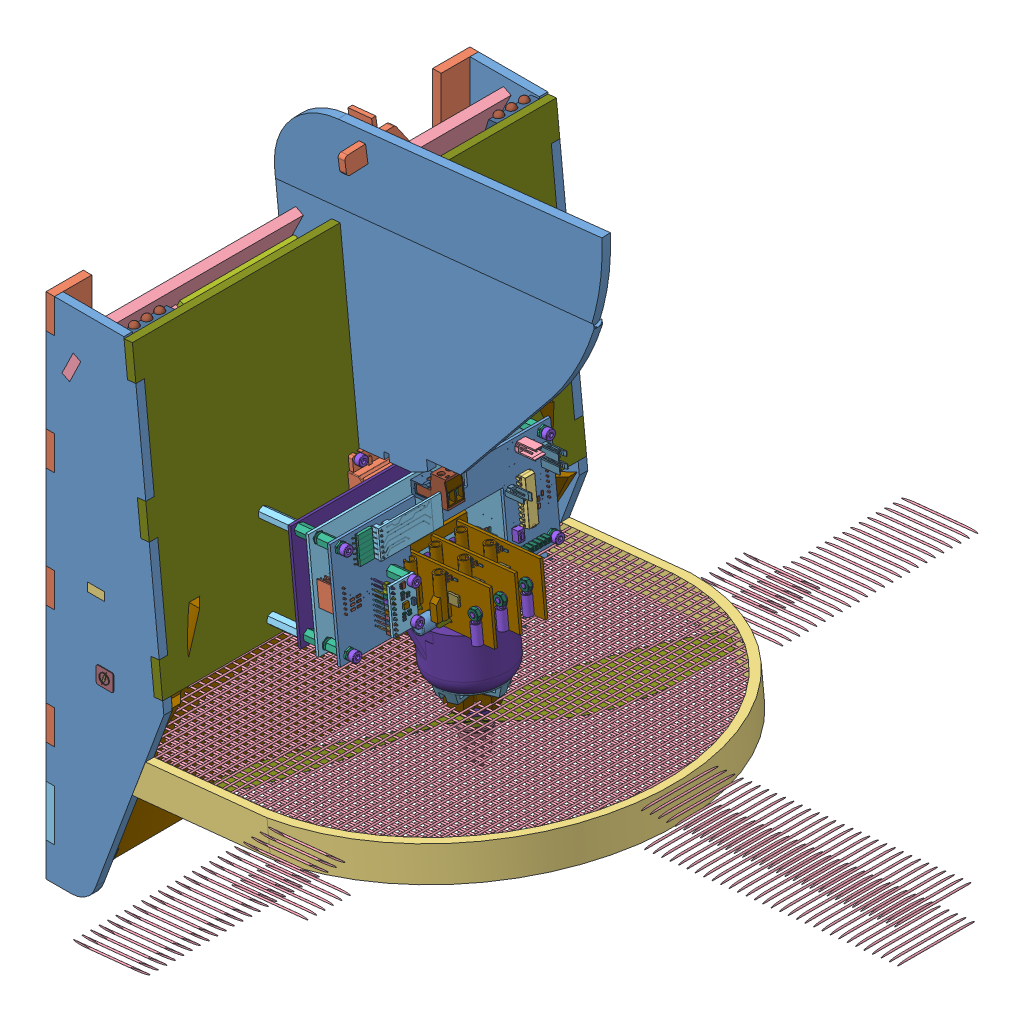
SolidWorks assembly AssTotale, configuration Défaut. Lengths in mm.
Overall size (253.25 376.61 251.6).
1718 component instances, 230 part files, 12 mates.
Components (placement in the parent):
- AssStructSimu-1: AssStructSimu [Défaut] at (-75.9431 -10.8604 24.5323) size (253.25 324.59 251.6)
  - AssBase-1: AssBase [Défaut] at (36.5482 -71.0398 34.0612) size (86.08 302.3 251.6)
    - AssD-1: AssD [Défaut] at (39.0992 31.0201 8.5) size (69.5 300 22)
      - P1-1: P1 [Défaut] at (-95.5819 194.6656 377.5) size (69.5 300 5)
      - P5-1: P5 [Défaut] at (-100.5819 -35.3344 360.5) x (0 1 0) z (1 0 0) size (230 22 5)
    - AssG-1: AssG [Défaut] at (39.0992 31.0201 -236.5) size (69.5 300 22)
      - P1-1: P1 [Défaut] at (-95.5819 194.6656 377.5) size (69.5 300 5)
      - P5-1: P5 [Défaut] at (-95.5819 -35.3344 399.5) x (0 1 0) z (-1 0 0) size (230 22 5)
    - P7-1: P7 [Défaut] at (-1.4828 89.6857 370.5) x (0 0 -1) z (0 -1 0) size (250 54.5 5)
    - P4-1: P4 [Défaut] at (-63.2363 165.9323 386) x (0 0 -1) z (0.898794 -0.438371 0) size (250 60.5 66.27)
    - P3-1: P3 [Défaut] at (-56.4828 -74.3143 146) x (0 0 1) z (-1 0 0) size (250 70 5)
    - P4b-1: P4b [Défaut] at (-58.7423 163.7404 190) x (0 0 1) z (0.438371 0.898794 0) size (152 56 2)
    - battery-1: battery [Défaut] at (-39.0156 204.1861 197.5) x (0 0 1) z (0.898794 -0.438371 0) size (137 43 30)
    - socket head cap screw 4762_din-1: socket head cap screw 4762_din [EN ISO 4762 M3 x 10 - 10N] at (-27.7008 145.2627 193) x (0.438371 0.898794 0) z (0 0 -1) size (13 5.5 5.5)
    - socket head cap screw 4762_din-2: socket head cap screw 4762_din [EN ISO 4762 M3 x 10 - 10N] at (-27.7008 145.2627 339) x (0.438371 0.898794 0) z (-0.791285 0.385936 -0.474259) size (13 5.5 5.5)
    - socket head cap screw 4762_din-3: socket head cap screw 4762_din [EN ISO 4762 M3 x 10 - 10N] at (-42.0815 152.2766 339) x (0.438371 0.898794 0) z (-0.001489 0.000726 -0.999999) size (13 5.5 5.5)
    - socket head cap screw 4762_din-4: socket head cap screw 4762_din [EN ISO 4762 M3 x 10 - 10N] at (-42.0815 152.2766 193) x (0.438371 0.898794 0) z (-0.031331 0.015281 -0.999392) size (13 5.5 5.5)
    - P11-1: P11 [Défaut] at (-57.5734 -73.9703 146.7843) x (0.005072 0 0.999987) z (0.006197 0.999981 -0.000031) size (240 65 164)
    - AssPhare-1: AssPhare [Défaut] at (-52.8518 -67.6977 411) x (0 1 0) z (0 0 -1) size (40.8 8 27.06)
      - piece_led-1: piece_led [Défaut] at (-6.6166 -3.631 25) size (7 8 25)
      - LED 5mm-1: LED 5mm [Valor predeterminado] at (-0.1166 0.369 30) x (0 0 1) z (-1 0 0) size (5.5 6 35.8)
      - LED 5mm-2: LED 5mm [Valor predeterminado] at (-0.1166 0.369 37.5) x (0 0 1) z (-1 0 0) size (5.5 6 35.8)
      - LED 5mm-3: LED 5mm [Valor predeterminado] at (-0.1166 0.369 45) x (0 0 1) z (-1 0 0) size (5.5 6 35.8)
    - AssPhare-2: AssPhare [Défaut] at (-52.8518 -67.6977 196) x (0 1 0) z (0 0 -1) size (40.8 8 27.06)
      - piece_led-1: piece_led [Défaut] at (-6.6166 -3.631 25) size (7 8 25)
      - LED 5mm-1: LED 5mm [Valor predeterminado] at (-0.1166 0.369 30) x (0 0 1) z (-1 0 0) size (5.5 6 35.8)
      - LED 5mm-2: LED 5mm [Valor predeterminado] at (-0.1166 0.369 37.5) x (0 0 1) z (-1 0 0) size (5.5 6 35.8)
      - LED 5mm-3: LED 5mm [Valor predeterminado] at (-0.1166 0.369 45) x (0 0 1) z (-1 0 0) size (5.5 6 35.8)
    - AssLogo-1: AssLogo [Défaut] at (-27.8835 45.1673 148.1054) x (-1 0 0) z (0 0 -1) size (10 10 0.8)
      - logo1-1: logo1 [Défaut] at (-6.5271 -4.4734 6.5054) size (5.8 7.71 0.4)
      - logo2-1: logo2 [Défaut] at (-6.4007 -4.4815 7.1054) size (10 10 0.4)
    - AssLogo-2: AssLogo [Défaut] at (-25.082 45.1673 383.8946) size (10 10 0.8)
      - logo1-1: logo1 [Défaut] at (-6.5271 -4.4734 6.5054) size (5.8 7.71 0.4)
      - logo2-1: logo2 [Défaut] at (-6.4007 -4.4815 7.1054) size (10 10 0.4)
    - support2-1: support2 [Défaut] at (-61.5648 191.7124 276) x (-0.017452 -0.999848 0) z (0.999848 -0.017452 0) size (75 20 10)
    - socket head cap screw 4762_din-5: socket head cap screw 4762_din [EN ISO 4762 M3 x 5 - 5N] at (-61.652 186.7132 269.3333) x (0.999848 -0.017452 0) z (-0.002158 -0.123615 0.992328) size (8 5.5 5.5)
    - socket head cap screw 4762_din-6: socket head cap screw 4762_din [EN ISO 4762 M3 x 5 - 5N] at (-61.652 186.7132 262.6667) x (0.999848 -0.017452 0) z (0 0 1) size (8 5.5 5.5)
    - socket head cap screw 4762_din-7: socket head cap screw 4762_din [EN ISO 4762 M3 x 25 - 18N] at (-55.2963 121.0922 253) x (0 0 1) z (-1 0 0) size (28 5.5 5.5)
    - hex nut style 1 gradeab_din-1: hex nut style 1 gradeab_din [Hexagon Nut ISO 4032 - M3 - W - N] at (-55.2963 121.0922 276) x (-0.923728 -0.383049 0) z (0 0 -1) size (5.5 6.35 2.4)
  - AssToitMot-1: AssToitMot [Défaut] at (-168.5238 43.6961 238.494) x (0 0 -1) z (0.9948 0.101852 0) size (250 207.5 205)
    - AssToit-1: AssToit [Défaut] at (-23.0702 -16.5789 -3.7148) size (250 207.5 205)
      - P8-1: P8 [Défaut] at (-38.4971 122.5921 203.5) size (250 175 5)
      - P12-1: P12 [Défaut] at (-60.4971 -63.4079 265.5) x (1 0 0) z (0 -1 0) size (47.03 76.64 55)
      - P13-1: P13 [Défaut] at (-35.9971 -52.8579 208.5) x (0 0 1) z (-1 0 0) size (64 15.55 5)
      - P10_2-1: P10_2 [Défaut] at (-35.9971 111.5921 171) x (0 0 1) z (-1 0 0) size (188.5 117.6 5)
    - Parallax-Servo_DUMMY-1: Parallax-Servo_DUMMY [Défaut] at (-61.6002 -51.5207 216.6662) x (1 0 0) z (0 1 0) size (20.07 42.67 55.64)
    - socket head cap screw 4762_din-1: socket head cap screw 4762_din [EN ISO 4762 M2.5 x 5 - 5N] at (-51.9272 -76.4868 259.2852) x (0 -1 0) z (-0.546944 0 0.837169) size (7.5 4.5 4.5)
    - socket head cap screw 4762_din-2: socket head cap screw 4762_din [EN ISO 4762 M2.5 x 5 - 5N] at (-61.5672 -76.4868 268.9252) x (0 -1 0) z (-0.546944 0 0.837169) size (7.5 4.5 4.5)
    - socket head cap screw 4762_din-3: socket head cap screw 4762_din [EN ISO 4762 M2.5 x 5 - 5N] at (-71.2072 -76.4868 259.2852) x (0 -1 0) z (-0.546944 0 0.837169) size (7.5 4.5 4.5)
    - socket head cap screw 4762_din-4: socket head cap screw 4762_din [EN ISO 4762 M2.5 x 5 - 5N] at (-61.5672 -76.4868 249.6452) x (0 -1 0) z (-0.546944 0 0.837169) size (7.5 4.5 4.5)
    - AssPhare-1: AssPhare [Défaut] at (8.4328 83.3966 196.1542) x (0 -1 0) z (1 0 0) size (40.8 8 27.06)
      - piece_led-1: piece_led [Défaut] at (-6.6166 -3.631 25) size (7 8 25)
      - LED 5mm-1: LED 5mm [Valor predeterminado] at (-0.1166 0.369 30) x (0 0 1) z (-1 0 0) size (5.5 6 35.8)
      - LED 5mm-2: LED 5mm [Valor predeterminado] at (-0.1166 0.369 37.5) x (0 0 1) z (-1 0 0) size (5.5 6 35.8)
      - LED 5mm-3: LED 5mm [Valor predeterminado] at (-0.1166 0.369 45) x (0 0 1) z (-1 0 0) size (5.5 6 35.8)
    - AssPhare-2: AssPhare [Défaut] at (-206.5672 83.3966 196.1542) x (0 -1 0) z (1 0 0) size (40.8 8 27.06)
      - piece_led-1: piece_led [Défaut] at (-6.6166 -3.631 25) size (7 8 25)
      - LED 5mm-1: LED 5mm [Valor predeterminado] at (-0.1166 0.369 30) x (0 0 1) z (-1 0 0) size (5.5 6 35.8)
      - LED 5mm-2: LED 5mm [Valor predeterminado] at (-0.1166 0.369 37.5) x (0 0 1) z (-1 0 0) size (5.5 6 35.8)
      - LED 5mm-3: LED 5mm [Valor predeterminado] at (-0.1166 0.369 45) x (0 0 1) z (-1 0 0) size (5.5 6 35.8)
    - socket head cap screw 4762_din-5: socket head cap screw 4762_din [EN ISO 4762 M3 x 10 - 10N] at (-67.0672 -22.9368 210.2852) x (0 0 -1) z (1 0 0) size (13 5.5 5.5)
    - socket head cap screw 4762_din-6: socket head cap screw 4762_din [EN ISO 4762 M3 x 10 - 10N] at (-56.0672 -72.9868 210.2852) x (0 0 -1) z (1 0 0) size (13 5.5 5.5)
    - socket head cap screw 4762_din-7: socket head cap screw 4762_din [EN ISO 4762 M3 x 10 - 10N] at (-67.0672 -72.9868 210.2852) x (0 0 -1) z (1 0 0) size (13 5.5 5.5)
    - socket head cap screw 4762_din-8: socket head cap screw 4762_din [EN ISO 4762 M3 x 10 - 10N] at (-56.0672 -22.9368 210.2852) x (0 0 -1) z (1 0 0) size (13 5.5 5.5)
    - hex nut style 1 gradeab_din-1: hex nut style 1 gradeab_din [Hexagon Nut ISO 4032 - M3 - W - N] at (-67.0672 -72.9868 197.3852) x (-0.923728 -0.383049 0) z (0 0 -1) size (5.5 6.35 2.4)
    - hex nut style 1 gradeab_din-2: hex nut style 1 gradeab_din [Hexagon Nut ISO 4032 - M3 - W - N] at (-56.0672 -72.9868 199.7852) size (5.5 6.35 2.4)
    - hex nut style 1 gradeab_din-3: hex nut style 1 gradeab_din [Hexagon Nut ISO 4032 - M3 - W - N] at (-67.0672 -22.9368 199.7852) size (5.5 6.35 2.4)
    - hex nut style 1 gradeab_din-4: hex nut style 1 gradeab_din [Hexagon Nut ISO 4032 - M3 - W - N] at (-56.0672 -22.9368 199.7852) size (5.5 6.35 2.4)
  - AssProtec-1: AssProtec [Défaut] at (86.6746 190.4649 284.6351) x (0 0 -1) z (0.101852 -0.9948 0) size (250 237.46 20)
    - protec3c-1: protec3c [Défaut] at (-140.4261 -87.7568 240) size (250 197 20)
    - AssGrillage-1: AssGrillage [Défaut] at (-370.4609 -132.5428 258.3161) x (0 0 -1) z (1 0 0) size (2.02 237.05 250)
      - barreau-1: barreau [Défaut] at (-1.1839 0.254 200) size (1 1 400)
      - barreau-3: barreau [Défaut] at (-1.1839 5.254 200) size (1 1 400)
      - barreau-4: barreau [Défaut] at (-1.1839 10.254 200) size (1 1 400)
      - barreau-5: barreau [Défaut] at (-1.1839 15.254 200) size (1 1 400)
      - barreau-6: barreau [Défaut] at (-1.1839 20.254 200) size (1 1 400)
      - barreau-7: barreau [Défaut] at (-1.1839 25.254 200) size (1 1 400)
      - barreau-8: barreau [Défaut] at (-1.1839 30.254 200) size (1 1 400)
      - barreau-9: barreau [Défaut] at (-1.1839 35.254 200) size (1 1 400)
      - barreau-10: barreau [Défaut] at (-1.1839 40.254 200) size (1 1 400)
      - barreau-11: barreau [Défaut] at (-1.1839 45.254 200) size (1 1 400)
      - barreau-12: barreau [Défaut] at (-1.1839 50.254 200) size (1 1 400)
      - barreau-13: barreau [Défaut] at (-1.1839 55.254 200) size (1 1 400)
      - barreau-14: barreau [Défaut] at (-1.1839 60.254 200) size (1 1 400)
      - barreau-15: barreau [Défaut] at (-1.1839 65.254 200) size (1 1 400)
      - barreau-16: barreau [Défaut] at (-1.1839 70.254 200) size (1 1 400)
      - barreau-17: barreau [Défaut] at (-1.1839 75.254 200) size (1 1 400)
      - barreau-18: barreau [Défaut] at (-1.1839 80.254 200) size (1 1 400)
      - barreau-19: barreau [Défaut] at (-1.1839 85.254 200) size (1 1 400)
      - barreau-20: barreau [Défaut] at (-1.1839 90.254 200) size (1 1 400)
      - barreau-21: barreau [Défaut] at (-1.1839 95.254 200) size (1 1 400)
      - barreau-22: barreau [Défaut] at (-1.1839 100.254 200) size (1 1 400)
      - barreau-23: barreau [Défaut] at (-1.1839 105.254 200) size (1 1 400)
      - barreau-24: barreau [Défaut] at (-1.1839 110.254 200) size (1 1 400)
      - barreau-25: barreau [Défaut] at (-1.1839 115.254 200) size (1 1 400)
      - barreau-26: barreau [Défaut] at (-1.1839 120.254 200) size (1 1 400)
      - barreau-27: barreau [Défaut] at (-1.1839 125.254 200) size (1 1 400)
      - barreau-28: barreau [Défaut] at (-1.1839 130.254 200) size (1 1 400)
      - barreau-29: barreau [Défaut] at (-1.1839 135.254 200) size (1 1 400)
      - barreau-30: barreau [Défaut] at (-1.1839 140.254 200) size (1 1 400)
      - barreau-31: barreau [Défaut] at (-1.1839 145.254 200) size (1 1 400)
      - barreau-32: barreau [Défaut] at (-1.1839 150.254 200) size (1 1 400)
      - barreau-33: barreau [Défaut] at (-1.1839 155.254 200) size (1 1 400)
      - barreau-34: barreau [Défaut] at (-1.1839 160.254 200) size (1 1 400)
      - barreau-35: barreau [Défaut] at (-1.1839 165.254 200) size (1 1 400)
      - barreau-36: barreau [Défaut] at (-1.1839 170.254 200) size (1 1 400)
      - barreau-37: barreau [Défaut] at (-1.1839 175.254 200) size (1 1 400)
      - barreau-38: barreau [Défaut] at (-1.1839 180.254 200) size (1 1 400)
      - barreau-39: barreau [Défaut] at (-1.1839 185.254 200) size (1 1 400)
      - barreau-40: barreau [Défaut] at (-1.1839 190.254 200) size (1 1 400)
      - barreau-41: barreau [Défaut] at (-1.1839 195.254 200) size (1 1 400)
      - barreau-42: barreau [Défaut] at (-0.1839 -1.5314 598.7823) x (0.998922 0 0.04641) z (0 1 0) size (1 1 400)
      - barreau-43: barreau [Défaut] at (-1.1839 200.254 200) size (1 1 400)
      - barreau-44: barreau [Défaut] at (-1.1839 205.254 200) size (1 1 400)
      - barreau-45: barreau [Défaut] at (-1.1839 210.254 200) size (1 1 400)
      - barreau-46: barreau [Défaut] at (-1.1839 215.254 200) size (1 1 400)
      - barreau-47: barreau [Défaut] at (-1.1839 220.254 200) size (1 1 400)
      - barreau-48: barreau [Défaut] at (-1.1839 225.254 200) size (1 1 400)
      - barreau-49: barreau [Défaut] at (-1.1839 230.254 200) size (1 1 400)
      - barreau-50: barreau [Défaut] at (-1.1839 235.254 200) size (1 1 400)
      - barreau-51: barreau [Défaut] at (-1.1839 240.254 200) size (1 1 400)
      - barreau-52: barreau [Défaut] at (-1.1839 245.254 200) size (1 1 400)
      - barreau-53: barreau [Défaut] at (-1.1839 250.254 200) size (1 1 400)
      - barreau-54: barreau [Défaut] at (-1.1839 255.254 200) size (1 1 400)
      - barreau-55: barreau [Défaut] at (-1.1839 260.254 200) size (1 1 400)
      - barreau-56: barreau [Défaut] at (-1.1839 265.254 200) size (1 1 400)
      - barreau-57: barreau [Défaut] at (-1.1839 270.254 200) size (1 1 400)
      - barreau-58: barreau [Défaut] at (-1.1839 275.254 200) size (1 1 400)
      - barreau-59: barreau [Défaut] at (-1.1839 280.254 200) size (1 1 400)
      - barreau-60: barreau [Défaut] at (-1.1839 285.254 200) size (1 1 400)
      - barreau-61: barreau [Défaut] at (-1.1839 290.254 200) size (1 1 400)
      - barreau-62: barreau [Défaut] at (-1.1839 295.254 200) size (1 1 400)
      - barreau-63: barreau [Défaut] at (-1.1839 300.254 200) size (1 1 400)
      - barreau-64: barreau [Défaut] at (-1.1839 305.254 200) size (1 1 400)
      - barreau-65: barreau [Défaut] at (-1.1839 310.254 200) size (1 1 400)
      - barreau-66: barreau [Défaut] at (-1.1839 315.254 200) size (1 1 400)
      - barreau-67: barreau [Défaut] at (-1.1839 320.254 200) size (1 1 400)
      - barreau-68: barreau [Défaut] at (-1.1839 325.254 200) size (1 1 400)
      - barreau-69: barreau [Défaut] at (-1.1839 330.254 200) size (1 1 400)
      - barreau-70: barreau [Défaut] at (-1.1839 335.254 200) size (1 1 400)
      - barreau-71: barreau [Défaut] at (-1.1839 340.254 200) size (1 1 400)
      - barreau-72: barreau [Défaut] at (-1.1839 345.254 200) size (1 1 400)
      - barreau-73: barreau [Défaut] at (-1.1839 350.254 200) size (1 1 400)
      - barreau-74: barreau [Défaut] at (-1.1839 355.254 200) size (1 1 400)
      - barreau-75: barreau [Défaut] at (-1.1839 360.254 200) size (1 1 400)
      - barreau-76: barreau [Défaut] at (-1.1839 365.254 200) size (1 1 400)
      - barreau-77: barreau [Défaut] at (-1.1839 370.254 200) size (1 1 400)
      - barreau-78: barreau [Défaut] at (-1.1839 375.254 200) size (1 1 400)
      - barreau-79: barreau [Défaut] at (-1.1839 380.254 200) size (1 1 400)
      - barreau-80: barreau [Défaut] at (-1.1839 385.254 200) size (1 1 400)
      - barreau-81: barreau [Défaut] at (-1.1839 390.254 200) size (1 1 400)
      - barreau-82: barreau [Défaut] at (-1.1839 395.254 200) size (1 1 400)
      - barreau-136: barreau [Défaut] at (-0.1839 -1.5314 593.7823) x (0.998922 0 0.04641) z (0 1 0) size (1 1 400)
      - barreau-137: barreau [Défaut] at (-0.1839 -1.5314 588.7823) x (0.998922 0 0.04641) z (0 1 0) size (1 1 400)
      - barreau-138: barreau [Défaut] at (-0.1839 -1.5314 583.7823) x (0.998922 0 0.04641) z (0 1 0) size (1 1 400)
      - barreau-139: barreau [Défaut] at (-0.1839 -1.5314 578.7823) x (0.998922 0 0.04641) z (0 1 0) size (1 1 400)
      - barreau-140: barreau [Défaut] at (-0.1839 -1.5314 573.7823) x (0.998922 0 0.04641) z (0 1 0) size (1 1 400)
      - barreau-141: barreau [Défaut] at (-0.1839 -1.5314 568.7823) x (0.998922 0 0.04641) z (0 1 0) size (1 1 400)
      - barreau-142: barreau [Défaut] at (-0.1839 -1.5314 563.7823) x (0.998922 0 0.04641) z (0 1 0) size (1 1 400)
      - barreau-143: barreau [Défaut] at (-0.1839 -1.5314 558.7823) x (0.998922 0 0.04641) z (0 1 0) size (1 1 400)
      - barreau-144: barreau [Défaut] at (-0.1839 -1.5314 553.7823) x (0.998922 0 0.04641) z (0 1 0) size (1 1 400)
      - barreau-145: barreau [Défaut] at (-0.1839 -1.5314 548.7823) x (0.998922 0 0.04641) z (0 1 0) size (1 1 400)
      - barreau-146: barreau [Défaut] at (-0.1839 -1.5314 543.7823) x (0.998922 0 0.04641) z (0 1 0) size (1 1 400)
      - barreau-147: barreau [Défaut] at (-0.1839 -1.5314 538.7823) x (0.998922 0 0.04641) z (0 1 0) size (1 1 400)
      - barreau-148: barreau [Défaut] at (-0.1839 -1.5314 533.7823) x (0.998922 0 0.04641) z (0 1 0) size (1 1 400)
      - barreau-149: barreau [Défaut] at (-0.1839 -1.5314 528.7823) x (0.998922 0 0.04641) z (0 1 0) size (1 1 400)
      - barreau-150: barreau [Défaut] at (-0.1839 -1.5314 523.7823) x (0.998922 0 0.04641) z (0 1 0) size (1 1 400)
      - barreau-151: barreau [Défaut] at (-0.1839 -1.5314 518.7823) x (0.998922 0 0.04641) z (0 1 0) size (1 1 400)
      - barreau-152: barreau [Défaut] at (-0.1839 -1.5314 513.7823) x (0.998922 0 0.04641) z (0 1 0) size (1 1 400)
      - barreau-153: barreau [Défaut] at (-0.1839 -1.5314 508.7823) x (0.998922 0 0.04641) z (0 1 0) size (1 1 400)
      - barreau-154: barreau [Défaut] at (-0.1839 -1.5314 503.7823) x (0.998922 0 0.04641) z (0 1 0) size (1 1 400)
      - barreau-155: barreau [Défaut] at (-0.1839 -1.5314 498.7823) x (0.998922 0 0.04641) z (0 1 0) size (1 1 400)
      - barreau-156: barreau [Défaut] at (-0.1839 -1.5314 493.7823) x (0.998922 0 0.04641) z (0 1 0) size (1 1 400)
      - barreau-157: barreau [Défaut] at (-0.1839 -1.5314 488.7823) x (0.998922 0 0.04641) z (0 1 0) size (1 1 400)
      - barreau-158: barreau [Défaut] at (-0.1839 -1.5314 483.7823) x (0.998922 0 0.04641) z (0 1 0) size (1 1 400)
      - barreau-159: barreau [Défaut] at (-0.1839 -1.5314 478.7823) x (0.998922 0 0.04641) z (0 1 0) size (1 1 400)
      - barreau-160: barreau [Défaut] at (-0.1839 -1.5314 473.7823) x (0.998922 0 0.04641) z (0 1 0) size (1 1 400)
      - barreau-161: barreau [Défaut] at (-0.1839 -1.5314 468.7823) x (0.998922 0 0.04641) z (0 1 0) size (1 1 400)
      - barreau-162: barreau [Défaut] at (-0.1839 -1.5314 463.7823) x (0.998922 0 0.04641) z (0 1 0) size (1 1 400)
      - barreau-163: barreau [Défaut] at (-0.1839 -1.5314 458.7823) x (0.998922 0 0.04641) z (0 1 0) size (1 1 400)
      - barreau-164: barreau [Défaut] at (-0.1839 -1.5314 453.7823) x (0.998922 0 0.04641) z (0 1 0) size (1 1 400)
      - barreau-165: barreau [Défaut] at (-0.1839 -1.5314 448.7823) x (0.998922 0 0.04641) z (0 1 0) size (1 1 400)
      - barreau-166: barreau [Défaut] at (-0.1839 -1.5314 443.7823) x (0.998922 0 0.04641) z (0 1 0) size (1 1 400)
      - barreau-167: barreau [Défaut] at (-0.1839 -1.5314 438.7823) x (0.998922 0 0.04641) z (0 1 0) size (1 1 400)
      - barreau-168: barreau [Défaut] at (-0.1839 -1.5314 433.7823) x (0.998922 0 0.04641) z (0 1 0) size (1 1 400)
      - barreau-169: barreau [Défaut] at (-0.1839 -1.5314 428.7823) x (0.998922 0 0.04641) z (0 1 0) size (1 1 400)
      - barreau-170: barreau [Défaut] at (-0.1839 -1.5314 423.7823) x (0.998922 0 0.04641) z (0 1 0) size (1 1 400)
      - barreau-171: barreau [Défaut] at (-0.1839 -1.5314 418.7823) x (0.998922 0 0.04641) z (0 1 0) size (1 1 400)
      - barreau-172: barreau [Défaut] at (-0.1839 -1.5314 413.7823) x (0.998922 0 0.04641) z (0 1 0) size (1 1 400)
      - barreau-173: barreau [Défaut] at (-0.1839 -1.5314 408.7823) x (0.998922 0 0.04641) z (0 1 0) size (1 1 400)
      - barreau-174: barreau [Défaut] at (-0.1839 -1.5314 403.7823) x (0.998922 0 0.04641) z (0 1 0) size (1 1 400)
      - barreau-175: barreau [Défaut] at (-0.1839 -1.5314 398.7823) x (0.998922 0 0.04641) z (0 1 0) size (1 1 400)
      - barreau-176: barreau [Défaut] at (-0.1839 -1.5314 393.7823) x (0.998922 0 0.04641) z (0 1 0) size (1 1 400)
      - barreau-177: barreau [Défaut] at (-0.1839 -1.5314 388.7823) x (0.998922 0 0.04641) z (0 1 0) size (1 1 400)
      - barreau-178: barreau [Défaut] at (-0.1839 -1.5314 383.7823) x (0.998922 0 0.04641) z (0 1 0) size (1 1 400)
      - barreau-179: barreau [Défaut] at (-0.1839 -1.5314 378.7823) x (0.998922 0 0.04641) z (0 1 0) size (1 1 400)
      - barreau-180: barreau [Défaut] at (-0.1839 -1.5314 373.7823) x (0.998922 0 0.04641) z (0 1 0) size (1 1 400)
      - barreau-181: barreau [Défaut] at (-0.1839 -1.5314 368.7823) x (0.998922 0 0.04641) z (0 1 0) size (1 1 400)
      - barreau-182: barreau [Défaut] at (-0.1839 -1.5314 363.7823) x (0.998922 0 0.04641) z (0 1 0) size (1 1 400)
      - barreau-183: barreau [Défaut] at (-0.1839 -1.5314 358.7823) x (0.998922 0 0.04641) z (0 1 0) size (1 1 400)
      - barreau-184: barreau [Défaut] at (-0.1839 -1.5314 353.7823) x (0.998922 0 0.04641) z (0 1 0) size (1 1 400)
      - barreau-185: barreau [Défaut] at (-0.1839 -1.5314 348.7823) x (0.998922 0 0.04641) z (0 1 0) size (1 1 400)
      - barreau-186: barreau [Défaut] at (-0.1839 -1.5314 343.7823) x (0.998922 0 0.04641) z (0 1 0) size (1 1 400)
      - barreau-187: barreau [Défaut] at (-0.1839 -1.5314 338.7823) x (0.998922 0 0.04641) z (0 1 0) size (1 1 400)
      - barreau-188: barreau [Défaut] at (-0.1839 -1.5314 333.7823) x (0.998922 0 0.04641) z (0 1 0) size (1 1 400)
      - barreau-189: barreau [Défaut] at (-0.1839 -1.5314 328.7823) x (0.998922 0 0.04641) z (0 1 0) size (1 1 400)
      - barreau-190: barreau [Défaut] at (-0.1839 -1.5314 323.7823) x (0.998922 0 0.04641) z (0 1 0) size (1 1 400)
      - barreau-191: barreau [Défaut] at (-0.1839 -1.5314 318.7823) x (0.998922 0 0.04641) z (0 1 0) size (1 1 400)
      - barreau-192: barreau [Défaut] at (-0.1839 -1.5314 313.7823) x (0.998922 0 0.04641) z (0 1 0) size (1 1 400)
      - barreau-193: barreau [Défaut] at (-0.1839 -1.5314 308.7823) x (0.998922 0 0.04641) z (0 1 0) size (1 1 400)
      - barreau-194: barreau [Défaut] at (-0.1839 -1.5314 303.7823) x (0.998922 0 0.04641) z (0 1 0) size (1 1 400)
      - barreau-195: barreau [Défaut] at (-0.1839 -1.5314 298.7823) x (0.998922 0 0.04641) z (0 1 0) size (1 1 400)
      - barreau-196: barreau [Défaut] at (-0.1839 -1.5314 293.7823) x (0.998922 0 0.04641) z (0 1 0) size (1 1 400)
      - barreau-197: barreau [Défaut] at (-0.1839 -1.5314 288.7823) x (0.998922 0 0.04641) z (0 1 0) size (1 1 400)
      - barreau-198: barreau [Défaut] at (-0.1839 -1.5314 283.7823) x (0.998922 0 0.04641) z (0 1 0) size (1 1 400)
      - barreau-199: barreau [Défaut] at (-0.1839 -1.5314 278.7823) x (0.998922 0 0.04641) z (0 1 0) size (1 1 400)
      - barreau-200: barreau [Défaut] at (-0.1839 -1.5314 273.7823) x (0.998922 0 0.04641) z (0 1 0) size (1 1 400)
      - barreau-201: barreau [Défaut] at (-0.1839 -1.5314 268.7823) x (0.998922 0 0.04641) z (0 1 0) size (1 1 400)
      - barreau-202: barreau [Défaut] at (-0.1839 -1.5314 263.7823) x (0.998922 0 0.04641) z (0 1 0) size (1 1 400)
      - barreau-203: barreau [Défaut] at (-0.1839 -1.5314 258.7823) x (0.998922 0 0.04641) z (0 1 0) size (1 1 400)
      - barreau-204: barreau [Défaut] at (-0.1839 -1.5314 253.7823) x (0.998922 0 0.04641) z (0 1 0) size (1 1 400)
      - barreau-205: barreau [Défaut] at (-0.1839 -1.5314 248.7823) x (0.998922 0 0.04641) z (0 1 0) size (1 1 400)
      - barreau-206: barreau [Défaut] at (-0.1839 -1.5314 243.7823) x (0.998922 0 0.04641) z (0 1 0) size (1 1 400)
      - barreau-207: barreau [Défaut] at (-0.1839 -1.5314 238.7823) x (0.998922 0 0.04641) z (0 1 0) size (1 1 400)
      - barreau-208: barreau [Défaut] at (-0.1839 -1.5314 233.7823) x (0.998922 0 0.04641) z (0 1 0) size (1 1 400)
      - barreau-209: barreau [Défaut] at (-0.1839 -1.5314 228.7823) x (0.998922 0 0.04641) z (0 1 0) size (1 1 400)
      - barreau-210: barreau [Défaut] at (-0.1839 -1.5314 223.7823) x (0.998922 0 0.04641) z (0 1 0) size (1 1 400)
      - barreau-211: barreau [Défaut] at (-0.1839 -1.5314 218.7823) x (0.998922 0 0.04641) z (0 1 0) size (1 1 400)
      - barreau-212: barreau [Défaut] at (-0.1839 -1.5314 213.7823) x (0.998922 0 0.04641) z (0 1 0) size (1 1 400)
      - barreau-213: barreau [Défaut] at (-0.1839 -1.5314 208.7823) x (0.998922 0 0.04641) z (0 1 0) size (1 1 400)
      - barreau-214: barreau [Défaut] at (-0.1839 -1.5314 203.7823) x (0.998922 0 0.04641) z (0 1 0) size (1 1 400)
    - AssGrillage-2: AssGrillage [Défaut] at (339.6086 -132.5428 241.6839) x (0 0 1) z (-1 0 0) size (2.02 237.05 250)
      - barreau-1: barreau [Défaut] at (-1.1839 0.254 200) size (1 1 400)
      - barreau-3: barreau [Défaut] at (-1.1839 5.254 200) size (1 1 400)
      - barreau-4: barreau [Défaut] at (-1.1839 10.254 200) size (1 1 400)
      - barreau-5: barreau [Défaut] at (-1.1839 15.254 200) size (1 1 400)
      - barreau-6: barreau [Défaut] at (-1.1839 20.254 200) size (1 1 400)
      - barreau-7: barreau [Défaut] at (-1.1839 25.254 200) size (1 1 400)
      - barreau-8: barreau [Défaut] at (-1.1839 30.254 200) size (1 1 400)
      - barreau-9: barreau [Défaut] at (-1.1839 35.254 200) size (1 1 400)
      - barreau-10: barreau [Défaut] at (-1.1839 40.254 200) size (1 1 400)
      - barreau-11: barreau [Défaut] at (-1.1839 45.254 200) size (1 1 400)
      - barreau-12: barreau [Défaut] at (-1.1839 50.254 200) size (1 1 400)
      - barreau-13: barreau [Défaut] at (-1.1839 55.254 200) size (1 1 400)
      - barreau-14: barreau [Défaut] at (-1.1839 60.254 200) size (1 1 400)
      - barreau-15: barreau [Défaut] at (-1.1839 65.254 200) size (1 1 400)
      - barreau-16: barreau [Défaut] at (-1.1839 70.254 200) size (1 1 400)
      - barreau-17: barreau [Défaut] at (-1.1839 75.254 200) size (1 1 400)
      - barreau-18: barreau [Défaut] at (-1.1839 80.254 200) size (1 1 400)
      - barreau-19: barreau [Défaut] at (-1.1839 85.254 200) size (1 1 400)
      - barreau-20: barreau [Défaut] at (-1.1839 90.254 200) size (1 1 400)
      - barreau-21: barreau [Défaut] at (-1.1839 95.254 200) size (1 1 400)
      - barreau-22: barreau [Défaut] at (-1.1839 100.254 200) size (1 1 400)
      - barreau-23: barreau [Défaut] at (-1.1839 105.254 200) size (1 1 400)
      - barreau-24: barreau [Défaut] at (-1.1839 110.254 200) size (1 1 400)
      - barreau-25: barreau [Défaut] at (-1.1839 115.254 200) size (1 1 400)
      - barreau-26: barreau [Défaut] at (-1.1839 120.254 200) size (1 1 400)
      - barreau-27: barreau [Défaut] at (-1.1839 125.254 200) size (1 1 400)
      - barreau-28: barreau [Défaut] at (-1.1839 130.254 200) size (1 1 400)
      - barreau-29: barreau [Défaut] at (-1.1839 135.254 200) size (1 1 400)
      - barreau-30: barreau [Défaut] at (-1.1839 140.254 200) size (1 1 400)
      - barreau-31: barreau [Défaut] at (-1.1839 145.254 200) size (1 1 400)
      - barreau-32: barreau [Défaut] at (-1.1839 150.254 200) size (1 1 400)
      - barreau-33: barreau [Défaut] at (-1.1839 155.254 200) size (1 1 400)
      - barreau-34: barreau [Défaut] at (-1.1839 160.254 200) size (1 1 400)
      - barreau-35: barreau [Défaut] at (-1.1839 165.254 200) size (1 1 400)
      - barreau-36: barreau [Défaut] at (-1.1839 170.254 200) size (1 1 400)
      - barreau-37: barreau [Défaut] at (-1.1839 175.254 200) size (1 1 400)
      - barreau-38: barreau [Défaut] at (-1.1839 180.254 200) size (1 1 400)
      - barreau-39: barreau [Défaut] at (-1.1839 185.254 200) size (1 1 400)
      - barreau-40: barreau [Défaut] at (-1.1839 190.254 200) size (1 1 400)
      - barreau-41: barreau [Défaut] at (-1.1839 195.254 200) size (1 1 400)
      - barreau-42: barreau [Défaut] at (-0.1839 -1.5314 598.7823) x (0.998922 0 0.04641) z (0 1 0) size (1 1 400)
      - barreau-43: barreau [Défaut] at (-1.1839 200.254 200) size (1 1 400)
      - barreau-44: barreau [Défaut] at (-1.1839 205.254 200) size (1 1 400)
      - barreau-45: barreau [Défaut] at (-1.1839 210.254 200) size (1 1 400)
      - barreau-46: barreau [Défaut] at (-1.1839 215.254 200) size (1 1 400)
      - barreau-47: barreau [Défaut] at (-1.1839 220.254 200) size (1 1 400)
      - barreau-48: barreau [Défaut] at (-1.1839 225.254 200) size (1 1 400)
      - barreau-49: barreau [Défaut] at (-1.1839 230.254 200) size (1 1 400)
      - barreau-50: barreau [Défaut] at (-1.1839 235.254 200) size (1 1 400)
      - barreau-51: barreau [Défaut] at (-1.1839 240.254 200) size (1 1 400)
      - barreau-52: barreau [Défaut] at (-1.1839 245.254 200) size (1 1 400)
      - barreau-53: barreau [Défaut] at (-1.1839 250.254 200) size (1 1 400)
      - barreau-54: barreau [Défaut] at (-1.1839 255.254 200) size (1 1 400)
      - barreau-55: barreau [Défaut] at (-1.1839 260.254 200) size (1 1 400)
      - barreau-56: barreau [Défaut] at (-1.1839 265.254 200) size (1 1 400)
      - barreau-57: barreau [Défaut] at (-1.1839 270.254 200) size (1 1 400)
      - barreau-58: barreau [Défaut] at (-1.1839 275.254 200) size (1 1 400)
      - barreau-59: barreau [Défaut] at (-1.1839 280.254 200) size (1 1 400)
      - barreau-60: barreau [Défaut] at (-1.1839 285.254 200) size (1 1 400)
      - barreau-61: barreau [Défaut] at (-1.1839 290.254 200) size (1 1 400)
      - barreau-62: barreau [Défaut] at (-1.1839 295.254 200) size (1 1 400)
      - barreau-63: barreau [Défaut] at (-1.1839 300.254 200) size (1 1 400)
      - barreau-64: barreau [Défaut] at (-1.1839 305.254 200) size (1 1 400)
      - barreau-65: barreau [Défaut] at (-1.1839 310.254 200) size (1 1 400)
      - barreau-66: barreau [Défaut] at (-1.1839 315.254 200) size (1 1 400)
      - barreau-67: barreau [Défaut] at (-1.1839 320.254 200) size (1 1 400)
      - barreau-68: barreau [Défaut] at (-1.1839 325.254 200) size (1 1 400)
      - barreau-69: barreau [Défaut] at (-1.1839 330.254 200) size (1 1 400)
      - barreau-70: barreau [Défaut] at (-1.1839 335.254 200) size (1 1 400)
      - barreau-71: barreau [Défaut] at (-1.1839 340.254 200) size (1 1 400)
      - barreau-72: barreau [Défaut] at (-1.1839 345.254 200) size (1 1 400)
      - barreau-73: barreau [Défaut] at (-1.1839 350.254 200) size (1 1 400)
      - barreau-74: barreau [Défaut] at (-1.1839 355.254 200) size (1 1 400)
      - barreau-75: barreau [Défaut] at (-1.1839 360.254 200) size (1 1 400)
      - barreau-76: barreau [Défaut] at (-1.1839 365.254 200) size (1 1 400)
      - barreau-77: barreau [Défaut] at (-1.1839 370.254 200) size (1 1 400)
      - barreau-78: barreau [Défaut] at (-1.1839 375.254 200) size (1 1 400)
      - barreau-79: barreau [Défaut] at (-1.1839 380.254 200) size (1 1 400)
      - barreau-80: barreau [Défaut] at (-1.1839 385.254 200) size (1 1 400)
      - barreau-81: barreau [Défaut] at (-1.1839 390.254 200) size (1 1 400)
      - barreau-82: barreau [Défaut] at (-1.1839 395.254 200) size (1 1 400)
      - barreau-136: barreau [Défaut] at (-0.1839 -1.5314 593.7823) x (0.998922 0 0.04641) z (0 1 0) size (1 1 400)
      - barreau-137: barreau [Défaut] at (-0.1839 -1.5314 588.7823) x (0.998922 0 0.04641) z (0 1 0) size (1 1 400)
      - barreau-138: barreau [Défaut] at (-0.1839 -1.5314 583.7823) x (0.998922 0 0.04641) z (0 1 0) size (1 1 400)
      - barreau-139: barreau [Défaut] at (-0.1839 -1.5314 578.7823) x (0.998922 0 0.04641) z (0 1 0) size (1 1 400)
      - barreau-140: barreau [Défaut] at (-0.1839 -1.5314 573.7823) x (0.998922 0 0.04641) z (0 1 0) size (1 1 400)
      - barreau-141: barreau [Défaut] at (-0.1839 -1.5314 568.7823) x (0.998922 0 0.04641) z (0 1 0) size (1 1 400)
      - barreau-142: barreau [Défaut] at (-0.1839 -1.5314 563.7823) x (0.998922 0 0.04641) z (0 1 0) size (1 1 400)
      - barreau-143: barreau [Défaut] at (-0.1839 -1.5314 558.7823) x (0.998922 0 0.04641) z (0 1 0) size (1 1 400)
      - barreau-144: barreau [Défaut] at (-0.1839 -1.5314 553.7823) x (0.998922 0 0.04641) z (0 1 0) size (1 1 400)
      - barreau-145: barreau [Défaut] at (-0.1839 -1.5314 548.7823) x (0.998922 0 0.04641) z (0 1 0) size (1 1 400)
      - barreau-146: barreau [Défaut] at (-0.1839 -1.5314 543.7823) x (0.998922 0 0.04641) z (0 1 0) size (1 1 400)
      - barreau-147: barreau [Défaut] at (-0.1839 -1.5314 538.7823) x (0.998922 0 0.04641) z (0 1 0) size (1 1 400)
      - barreau-148: barreau [Défaut] at (-0.1839 -1.5314 533.7823) x (0.998922 0 0.04641) z (0 1 0) size (1 1 400)
      - barreau-149: barreau [Défaut] at (-0.1839 -1.5314 528.7823) x (0.998922 0 0.04641) z (0 1 0) size (1 1 400)
      - barreau-150: barreau [Défaut] at (-0.1839 -1.5314 523.7823) x (0.998922 0 0.04641) z (0 1 0) size (1 1 400)
      - barreau-151: barreau [Défaut] at (-0.1839 -1.5314 518.7823) x (0.998922 0 0.04641) z (0 1 0) size (1 1 400)
      - barreau-152: barreau [Défaut] at (-0.1839 -1.5314 513.7823) x (0.998922 0 0.04641) z (0 1 0) size (1 1 400)
      - barreau-153: barreau [Défaut] at (-0.1839 -1.5314 508.7823) x (0.998922 0 0.04641) z (0 1 0) size (1 1 400)
      - barreau-154: barreau [Défaut] at (-0.1839 -1.5314 503.7823) x (0.998922 0 0.04641) z (0 1 0) size (1 1 400)
      - barreau-155: barreau [Défaut] at (-0.1839 -1.5314 498.7823) x (0.998922 0 0.04641) z (0 1 0) size (1 1 400)
      - barreau-156: barreau [Défaut] at (-0.1839 -1.5314 493.7823) x (0.998922 0 0.04641) z (0 1 0) size (1 1 400)
      - barreau-157: barreau [Défaut] at (-0.1839 -1.5314 488.7823) x (0.998922 0 0.04641) z (0 1 0) size (1 1 400)
      - barreau-158: barreau [Défaut] at (-0.1839 -1.5314 483.7823) x (0.998922 0 0.04641) z (0 1 0) size (1 1 400)
      - barreau-159: barreau [Défaut] at (-0.1839 -1.5314 478.7823) x (0.998922 0 0.04641) z (0 1 0) size (1 1 400)
      - barreau-160: barreau [Défaut] at (-0.1839 -1.5314 473.7823) x (0.998922 0 0.04641) z (0 1 0) size (1 1 400)
      - barreau-161: barreau [Défaut] at (-0.1839 -1.5314 468.7823) x (0.998922 0 0.04641) z (0 1 0) size (1 1 400)
      - barreau-162: barreau [Défaut] at (-0.1839 -1.5314 463.7823) x (0.998922 0 0.04641) z (0 1 0) size (1 1 400)
      - barreau-163: barreau [Défaut] at (-0.1839 -1.5314 458.7823) x (0.998922 0 0.04641) z (0 1 0) size (1 1 400)
      - barreau-164: barreau [Défaut] at (-0.1839 -1.5314 453.7823) x (0.998922 0 0.04641) z (0 1 0) size (1 1 400)
      - barreau-165: barreau [Défaut] at (-0.1839 -1.5314 448.7823) x (0.998922 0 0.04641) z (0 1 0) size (1 1 400)
      - barreau-166: barreau [Défaut] at (-0.1839 -1.5314 443.7823) x (0.998922 0 0.04641) z (0 1 0) size (1 1 400)
      - barreau-167: barreau [Défaut] at (-0.1839 -1.5314 438.7823) x (0.998922 0 0.04641) z (0 1 0) size (1 1 400)
      - barreau-168: barreau [Défaut] at (-0.1839 -1.5314 433.7823) x (0.998922 0 0.04641) z (0 1 0) size (1 1 400)
      - barreau-169: barreau [Défaut] at (-0.1839 -1.5314 428.7823) x (0.998922 0 0.04641) z (0 1 0) size (1 1 400)
      - barreau-170: barreau [Défaut] at (-0.1839 -1.5314 423.7823) x (0.998922 0 0.04641) z (0 1 0) size (1 1 400)
      - barreau-171: barreau [Défaut] at (-0.1839 -1.5314 418.7823) x (0.998922 0 0.04641) z (0 1 0) size (1 1 400)
      - barreau-172: barreau [Défaut] at (-0.1839 -1.5314 413.7823) x (0.998922 0 0.04641) z (0 1 0) size (1 1 400)
      - barreau-173: barreau [Défaut] at (-0.1839 -1.5314 408.7823) x (0.998922 0 0.04641) z (0 1 0) size (1 1 400)
      - barreau-174: barreau [Défaut] at (-0.1839 -1.5314 403.7823) x (0.998922 0 0.04641) z (0 1 0) size (1 1 400)
      - barreau-175: barreau [Défaut] at (-0.1839 -1.5314 398.7823) x (0.998922 0 0.04641) z (0 1 0) size (1 1 400)
      - barreau-176: barreau [Défaut] at (-0.1839 -1.5314 393.7823) x (0.998922 0 0.04641) z (0 1 0) size (1 1 400)
      - barreau-177: barreau [Défaut] at (-0.1839 -1.5314 388.7823) x (0.998922 0 0.04641) z (0 1 0) size (1 1 400)
      - barreau-178: barreau [Défaut] at (-0.1839 -1.5314 383.7823) x (0.998922 0 0.04641) z (0 1 0) size (1 1 400)
      - barreau-179: barreau [Défaut] at (-0.1839 -1.5314 378.7823) x (0.998922 0 0.04641) z (0 1 0) size (1 1 400)
      - barreau-180: barreau [Défaut] at (-0.1839 -1.5314 373.7823) x (0.998922 0 0.04641) z (0 1 0) size (1 1 400)
      - barreau-181: barreau [Défaut] at (-0.1839 -1.5314 368.7823) x (0.998922 0 0.04641) z (0 1 0) size (1 1 400)
      - barreau-182: barreau [Défaut] at (-0.1839 -1.5314 363.7823) x (0.998922 0 0.04641) z (0 1 0) size (1 1 400)
      - barreau-183: barreau [Défaut] at (-0.1839 -1.5314 358.7823) x (0.998922 0 0.04641) z (0 1 0) size (1 1 400)
      - barreau-184: barreau [Défaut] at (-0.1839 -1.5314 353.7823) x (0.998922 0 0.04641) z (0 1 0) size (1 1 400)
      - barreau-185: barreau [Défaut] at (-0.1839 -1.5314 348.7823) x (0.998922 0 0.04641) z (0 1 0) size (1 1 400)
      - barreau-186: barreau [Défaut] at (-0.1839 -1.5314 343.7823) x (0.998922 0 0.04641) z (0 1 0) size (1 1 400)
      - barreau-187: barreau [Défaut] at (-0.1839 -1.5314 338.7823) x (0.998922 0 0.04641) z (0 1 0) size (1 1 400)
      - barreau-188: barreau [Défaut] at (-0.1839 -1.5314 333.7823) x (0.998922 0 0.04641) z (0 1 0) size (1 1 400)
      - barreau-189: barreau [Défaut] at (-0.1839 -1.5314 328.7823) x (0.998922 0 0.04641) z (0 1 0) size (1 1 400)
      - barreau-190: barreau [Défaut] at (-0.1839 -1.5314 323.7823) x (0.998922 0 0.04641) z (0 1 0) size (1 1 400)
      - barreau-191: barreau [Défaut] at (-0.1839 -1.5314 318.7823) x (0.998922 0 0.04641) z (0 1 0) size (1 1 400)
      - barreau-192: barreau [Défaut] at (-0.1839 -1.5314 313.7823) x (0.998922 0 0.04641) z (0 1 0) size (1 1 400)
      - barreau-193: barreau [Défaut] at (-0.1839 -1.5314 308.7823) x (0.998922 0 0.04641) z (0 1 0) size (1 1 400)
      - barreau-194: barreau [Défaut] at (-0.1839 -1.5314 303.7823) x (0.998922 0 0.04641) z (0 1 0) size (1 1 400)
      - barreau-195: barreau [Défaut] at (-0.1839 -1.5314 298.7823) x (0.998922 0 0.04641) z (0 1 0) size (1 1 400)
      - barreau-196: barreau [Défaut] at (-0.1839 -1.5314 293.7823) x (0.998922 0 0.04641) z (0 1 0) size (1 1 400)
      - barreau-197: barreau [Défaut] at (-0.1839 -1.5314 288.7823) x (0.998922 0 0.04641) z (0 1 0) size (1 1 400)
      - barreau-198: barreau [Défaut] at (-0.1839 -1.5314 283.7823) x (0.998922 0 0.04641) z (0 1 0) size (1 1 400)
      - barreau-199: barreau [Défaut] at (-0.1839 -1.5314 278.7823) x (0.998922 0 0.04641) z (0 1 0) size (1 1 400)
      - barreau-200: barreau [Défaut] at (-0.1839 -1.5314 273.7823) x (0.998922 0 0.04641) z (0 1 0) size (1 1 400)
      - barreau-201: barreau [Défaut] at (-0.1839 -1.5314 268.7823) x (0.998922 0 0.04641) z (0 1 0) size (1 1 400)
      - barreau-202: barreau [Défaut] at (-0.1839 -1.5314 263.7823) x (0.998922 0 0.04641) z (0 1 0) size (1 1 400)
      - barreau-203: barreau [Défaut] at (-0.1839 -1.5314 258.7823) x (0.998922 0 0.04641) z (0 1 0) size (1 1 400)
      - barreau-204: barreau [Défaut] at (-0.1839 -1.5314 253.7823) x (0.998922 0 0.04641) z (0 1 0) size (1 1 400)
      - barreau-205: barreau [Défaut] at (-0.1839 -1.5314 248.7823) x (0.998922 0 0.04641) z (0 1 0) size (1 1 400)
      - barreau-206: barreau [Défaut] at (-0.1839 -1.5314 243.7823) x (0.998922 0 0.04641) z (0 1 0) size (1 1 400)
      - barreau-207: barreau [Défaut] at (-0.1839 -1.5314 238.7823) x (0.998922 0 0.04641) z (0 1 0) size (1 1 400)
      - barreau-208: barreau [Défaut] at (-0.1839 -1.5314 233.7823) x (0.998922 0 0.04641) z (0 1 0) size (1 1 400)
      - barreau-209: barreau [Défaut] at (-0.1839 -1.5314 228.7823) x (0.998922 0 0.04641) z (0 1 0) size (1 1 400)
      - barreau-210: barreau [Défaut] at (-0.1839 -1.5314 223.7823) x (0.998922 0 0.04641) z (0 1 0) size (1 1 400)
      - barreau-211: barreau [Défaut] at (-0.1839 -1.5314 218.7823) x (0.998922 0 0.04641) z (0 1 0) size (1 1 400)
      - barreau-212: barreau [Défaut] at (-0.1839 -1.5314 213.7823) x (0.998922 0 0.04641) z (0 1 0) size (1 1 400)
      - barreau-213: barreau [Défaut] at (-0.1839 -1.5314 208.7823) x (0.998922 0 0.04641) z (0 1 0) size (1 1 400)
      - barreau-214: barreau [Défaut] at (-0.1839 -1.5314 203.7823) x (0.998922 0 0.04641) z (0 1 0) size (1 1 400)
  - AssCarte-1: AssCarte [Défaut] at (-42.8534 32.2132 302.028) x (-0.101852 0.9948 0) z (0.9948 0.101852 0) size (67.15 130.57 98.45)
    - carte_onduleur_v4-1: carte_onduleur_v4 [Défaut] at (-25.7639 0.8332 112.9379) size (66.52 130.57 82.34)
      - Layer_1-1: Layer_1 [Défaut] at origin size (60 130 1.61)
      - BTN-1: BTN [Défaut] at (-25.5 7.4 0.803) x (0 -1 0) z (0 0 1) size (6.76 3.64 4.37)
        - Open CASCADE STEP translator 6.8 1.2.1-1: Open CASCADE STEP translator 6.8 1.2.1 [Défaut] at origin size (6.76 3.64 4.37)
          - Body_1-1: Body_1 [Défaut] at (-0.5 -2 0) size (6.76 3.64 4.37)
            - =_[0_1_1_3]-1: =_[0_1_1_3] [Défaut] at origin size (6 3.64 4.37)
            - =_[0_1_1_4]-1: =_[0_1_1_4] [Défaut] at origin size (0.38 1 0.67)
            - =_[0_1_1_5]-1: =_[0_1_1_5] [Défaut] at origin size (0.38 1 0.67)
      - CON_IO1-1: CON_IO1 [Défaut] at (-11.3 12.1 0.803) x (0 -1 0) z (0 0 1) size (16.74 30.7 57.5)
        - Open CASCADE STEP translator 6.8 1.3.1-1: Open CASCADE STEP translator 6.8 1.3.1 [Défaut] at origin size (16.74 30.7 57.5)
          - Body_1_2-1: Body_1_2 [Défaut] at (-3 -15 8) x (0 -1 0) z (-1 0 0) size (30.7 57.5 16.74)
            - 1-1: 1 [Défaut] at origin size (30 50 1.61)
            - 10-1: 10 [Défaut] at (-14.395 31.0465 0.803) x (-1 0 0) z (0 0 1) size (5.59 6.35 1.11)
              - =_[0_1_1_4]-1: =_[0_1_1_4] [Défaut] at origin size (5.59 6.35 1.11)
                - 11-1: 11 [Défaut] at (2 3.3 0) x (-1 0 0) z (0 0 1) size (5.59 6.35 1.11)
                  - =_[0_1_1_3]_2-1: =_[0_1_1_3]_2 [Défaut] at origin size (0.44 0.55 0.36)
                  - =_[0_1_1_4]_2-1: =_[0_1_1_4]_2 [Défaut] at origin size (5.59 4.15 0.36)
                  - =_[0_1_1_5]_2-1: =_[0_1_1_5]_2 [Défaut] at origin size (5.35 6.1 1.1)
                  - =_[0_1_1_6]-1: =_[0_1_1_6] [Défaut] at origin size (0.44 0.55 0.36)
                  - =_[0_1_1_7]-1: =_[0_1_1_7] [Défaut] at origin size (0.44 0.55 0.36)
                  - =_[0_1_1_8]-1: =_[0_1_1_8] [Défaut] at origin size (0.44 0.55 0.36)
            - 13-1: 13 [Défaut] at (-12.62 16.6 -0.803) x (-1 0 0) z (0 0 -1) size (5.59 6.35 1.11)
              - =_[0_1_1_13]-1: =_[0_1_1_13] [Défaut] at origin size (5.59 6.35 1.11)
                - 11-1: 11 [Défaut] at (2 3.3 0) x (-1 0 0) z (0 0 1) size (5.59 6.35 1.11)
                  - =_[0_1_1_3]_2-1: =_[0_1_1_3]_2 [Défaut] at origin size (0.44 0.55 0.36)
                  - =_[0_1_1_4]_2-1: =_[0_1_1_4]_2 [Défaut] at origin size (5.59 4.15 0.36)
                  - =_[0_1_1_5]_2-1: =_[0_1_1_5]_2 [Défaut] at origin size (5.35 6.1 1.1)
                  - =_[0_1_1_6]-1: =_[0_1_1_6] [Défaut] at origin size (0.44 0.55 0.36)
                  - =_[0_1_1_7]-1: =_[0_1_1_7] [Défaut] at origin size (0.44 0.55 0.36)
                  - =_[0_1_1_8]-1: =_[0_1_1_8] [Défaut] at origin size (0.44 0.55 0.36)
            - 16-1: 16 [Défaut] at (-4.2 24.2 0.803) x (-1 0 0) z (0 0 1) size (12.8 0.5 13)
              - =_[0_1_1_15]-1: =_[0_1_1_15] [Défaut] at origin size (12.8 0.5 13)
                - 17-1: 17 [Défaut] at (2.7 0 0) x (1 0 0) z (0 -1 0) size (12.8 13 0.5)
            - 19-1: 19 [Défaut] at (-4.1 6.8 0.803) x (-1 0 0) z (0 0 1) size (12.8 0.5 13)
              - =_[0_1_1_18]-1: =_[0_1_1_18] [Défaut] at origin size (12.8 0.5 13)
                - 17-1: 17 [Défaut] at (2.7 0 0) x (1 0 0) z (0 -1 0) size (12.8 13 0.5)
            - 24-1: 24 [Défaut] at (-8.1 16.5 -0.803) x (0 1 0) z (0 0 -1) size (7.75 5.13 1.17)
              - =_[0_1_1_20]-1: =_[0_1_1_20] [Défaut] at origin size (7.75 5.13 1.17)
                - 20-1: 20 [Défaut] at origin size (7.59 5.13 1.07)
                - 21-1: 21 [Défaut] at (-14.478 0 0) x (-1 0 0) z (0 0 1) size (0.76 5.08 1.17)
                - 22-1: 22 [Défaut] at origin size (0.76 5.08 1.17)
            - 35-1: 35 [Défaut] at (-25.3 25.5 0.803) x (0 -1 0) z (0 0 1) size (6.05 5.2 1.7)
              - =_[0_1_1_25]-1: =_[0_1_1_25] [Défaut] at origin size (6.05 5.2 1.7)
                - 25-1: 25 [Défaut] at origin size (4.3 5.2 1.53)
                - 26-1: 26 [Défaut] at origin size (0.88 0.51 1.06)
                - 27-1: 27 [Défaut] at origin size (0.88 0.51 1.06)
                - 28-1: 28 [Défaut] at origin size (0.88 0.51 1.06)
                - 29-1: 29 [Défaut] at origin size (0.88 0.51 1.06)
                - 30-1: 30 [Défaut] at (11.6 -5.08 0) x (-1 0 0) z (0 0 1) size (0.87 0.51 1.06)
                - 31-1: 31 [Défaut] at (11.6 -2.54 0) x (-1 0 0) z (0 0 1) size (0.87 0.51 1.06)
                - 32-1: 32 [Défaut] at (11.6 0 0) x (-1 0 0) z (0 0 1) size (0.87 0.51 1.06)
                - 33-1: 33 [Défaut] at (11.6 2.54 0) x (-1 0 0) z (0 0 1) size (0.87 0.51 1.06)
            - 40-1: 40 [Défaut] at (-27.6 27.2 0.803) size (2.34 1.04 0.5)
              - =_[0_1_1_36]-1: =_[0_1_1_36] [Défaut] at origin size (2.34 1.04 0.5)
                - 36-1: 36 [Défaut] at origin size (2.29 1.04 0.43)
                - 37-1: 37 [Défaut] at (0.3048 0 0) x (-1 0 0) z (0 0 1) size (0.51 1.02 0.5)
                - 38-1: 38 [Défaut] at origin size (0.51 1.02 0.5)
            - 42-1: 42 [Défaut] at (-22.1 21.6 0.803) x (0 1 0) z (0 0 1) size (2.34 1.04 0.5)
              - =_[0_1_1_36]-1: =_[0_1_1_36] [Défaut] at origin size (2.34 1.04 0.5)
                - 36-1: 36 [Défaut] at origin size (2.29 1.04 0.43)
                - 37-1: 37 [Défaut] at (0.3048 0 0) x (-1 0 0) z (0 0 1) size (0.51 1.02 0.5)
                - 38-1: 38 [Défaut] at origin size (0.51 1.02 0.5)
            - 47-1: 47 [Défaut] at (-14.7664 14.5 -0.803) x (-1 0 0) z (0 0 -1) size (2.34 1.04 0.5)
              - =_[0_1_1_42]-1: =_[0_1_1_42] [Défaut] at origin size (2.34 1.04 0.5)
                - 43-1: 43 [Défaut] at origin size (2.29 1.04 0.43)
                - 44-1: 44 [Défaut] at (0.3048 0 0) x (-1 0 0) z (0 0 1) size (0.51 1.02 0.5)
                - 45-1: 45 [Défaut] at origin size (0.51 1.02 0.5)
            - 57-1: 57 [Défaut] at (-15.3 2.7 -0.803) x (0 -1 0) z (0 0 -1) size (10.36 15.24 6.14)
              - =_[0_1_1_47]-1: =_[0_1_1_47] [Défaut] at origin size (10.36 15.24 6.14)
                - 55-1: 55 [Défaut] at (1.8 -1.2 3) x (1 0 0) z (0 1 0) size (10.36 6.14 15.24)
                  - 54-1: 54 [Défaut] at origin size (10.36 6.14 7.62)
                    - 52-1: 52 [Défaut] at origin size (10.36 6.14 2.54)
                      - 48-1: 48 [Défaut] at origin size (8.4 2.54 2.54)
                      - 49-1: 49 [Défaut] at (-0.0461 1.2682 1.27) x (0 0 -1) z (0.999998 -0.002105 0) size (1.95 5.07 7.58)
                    - 52-2: 52 [Défaut] at (0 0 -2.54) size (10.36 6.14 2.54)
                      - 48-1: 48 [Défaut] at origin size (8.4 2.54 2.54)
                      - 49-1: 49 [Défaut] at (-0.0461 1.2682 1.27) x (0 0 -1) z (0.999998 -0.002105 0) size (1.95 5.07 7.58)
                    - 52-3: 52 [Défaut] at (0 0 -5.08) size (10.36 6.14 2.54)
                      - 48-1: 48 [Défaut] at origin size (8.4 2.54 2.54)
                      - 49-1: 49 [Défaut] at (-0.0461 1.2682 1.27) x (0 0 -1) z (0.999998 -0.002105 0) size (1.95 5.07 7.58)
                  - 54-2: 54 [Défaut] at (0 0 -7.62) size (10.36 6.14 7.62)
                    - 52-1: 52 [Défaut] at origin size (10.36 6.14 2.54)
                      - 48-1: 48 [Défaut] at origin size (8.4 2.54 2.54)
                      - 49-1: 49 [Défaut] at (-0.0461 1.2682 1.27) x (0 0 -1) z (0.999998 -0.002105 0) size (1.95 5.07 7.58)
                    - 52-2: 52 [Défaut] at (0 0 -2.54) size (10.36 6.14 2.54)
